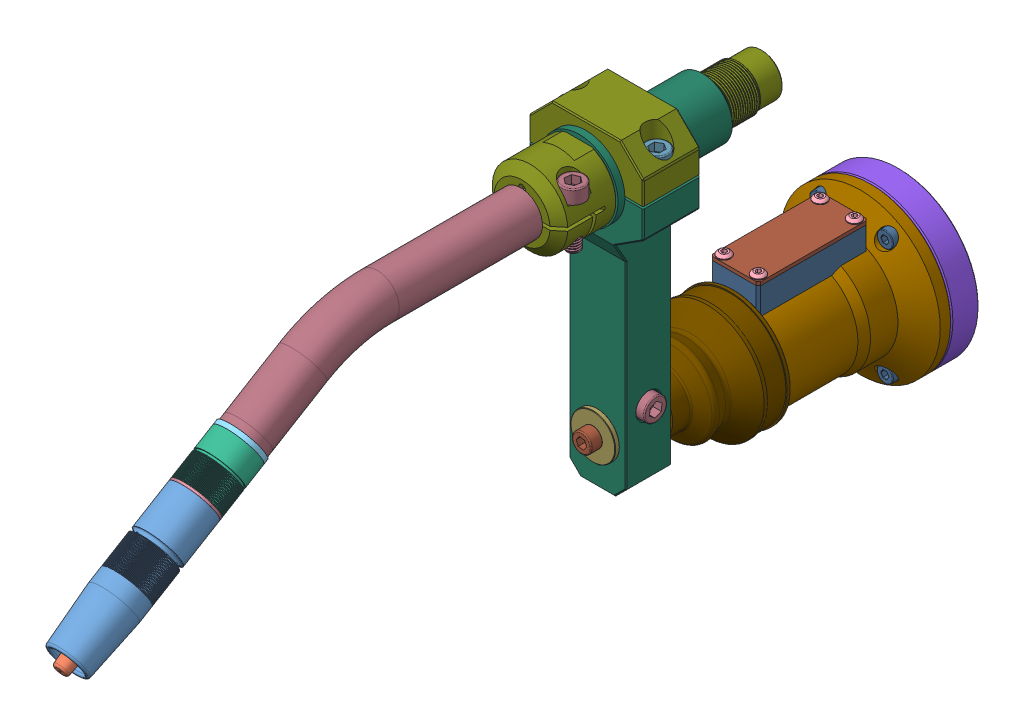
SolidWorks assembly 31度鵝頸，支架100.5L, configuration 默认. Lengths in mm.
Overall size (70 159.03 372.5).
47 component instances, 34 part files, 0 mates.
Components (placement in the parent):
- 31度鵝頸，支架100.5L-Part-1-1: 31度鵝頸，支架100.5L-Part-1 [默认] at (-1.3223 63.2513 288.8466) x (1 0 0) z (0 -0.857167 -0.515038) size (20 65.51 20)
- 31度鵝頸，支架100.5L-Part-2-1: 31度鵝頸，支架100.5L-Part-2 [默认] at (-1.3223 48.8303 312.8473) x (0 -0.515038 0.857167) z (-0.857167 0.441474 0.265264) size (40.5 8.7 8.7)
- 31度鵝頸，支架100.5L-Part-3-1: 31度鵝頸，支架100.5L-Part-3 [默认] at (-1.3223 56.2983 300.4183) x (1 0 0) z (0 -0.857167 -0.515038) size (15.5 21 15.5)
- 31度鵝頸，支架100.5L-Part-4-1: 31度鵝頸，支架100.5L-Part-4 [默认] at (-1.3223 63.7664 287.9894) x (0.857167 -0.441474 -0.265264) z (0 -0.515038 0.857167) size (20 20 1)
- 31度鵝頸，支架100.5L-Part-4-2: 31度鵝頸，支架100.5L-Part-4 [默认] at (-1.3223 63.2513 288.8466) x (1 0 0) z (0 0.515038 -0.857167) size (20 20 1)
- 31度鵝頸，支架100.5L-Part-5-1: 31度鵝頸，支架100.5L-Part-5 [默认] at (-1.3223 76.3848 266.9888) x (0 -0.515038 0.857167) z (-0.857167 0.441474 0.265264) size (38 20 20)
- 31度鵝頸，支架100.5L-Part-6-1: 31度鵝頸，支架100.5L-Part-6 [默认] at (-1.3223 76.3848 266.9888) x (0 -0.515038 0.857167) z (-0.857167 0.441474 0.265264) size (33.02 20 20)
- 31度鵝頸，支架100.5L-Part-7-1: 31度鵝頸，支架100.5L-Part-7 [默认] at (-1.3223 44.9675 319.276) x (0 0.515038 -0.857167) z (0.857167 0.441474 0.265264) size (80 14 16)
- 31度鵝頸，支架100.5L-Part-8-1: 31度鵝頸，支架100.5L-Part-8 [默认] at (-1.3223 100.8266 121.034) x (0 0 -1) z (1 0 0) size (2 12 12)
- 31度鵝頸，支架100.5L-Part-9-1: 31度鵝頸，支架100.5L-Part-9 [默认] at (-1.3223 0.3266 10.634) x (0 0 -1) z (-1 0 0) size (20 70 70)
- 31度鵝頸，支架100.5L-Part-10-1: 31度鵝頸，支架100.5L-Part-10 [默认] at (-16.0584 25.8771 1.634) x (-1 0 0) z (0 0 1) size (7 7 19)
- 31度鵝頸，支架100.5L-Part-10-2: 31度鵝頸，支架100.5L-Part-10 [默认] at (13.4416 25.8771 1.634) x (-1 0 0) z (0 0 1) size (7 7 19)
- 31度鵝頸，支架100.5L-Part-10-3: 31度鵝頸，支架100.5L-Part-10 [默认] at (-30.8084 0.3294 1.634) x (-1 0 0) z (0 0 1) size (7 7 19)
- 31度鵝頸，支架100.5L-Part-10-4: 31度鵝頸，支架100.5L-Part-10 [默认] at (13.4416 -25.2184 1.634) x (-1 0 0) z (0 0 1) size (7 7 19)
- 31度鵝頸，支架100.5L-Part-10-5: 31度鵝頸，支架100.5L-Part-10 [默认] at (-16.0584 -25.2184 1.634) x (-1 0 0) z (0 0 1) size (7 7 19)
- 31度鵝頸，支架100.5L-Part-11-1: 31度鵝頸，支架100.5L-Part-11 [默认] at (-1.3223 0.3266 119.534) x (0.923728 0.383049 0) z (0 0 -1) size (8.5 8.5 13.05)
- 31度鵝頸，支架100.5L-Part-12-1: 31度鵝頸，支架100.5L-Part-12 [默认] at (-1.3223 0.3266 114.534) x (-0.923728 -0.383049 0) z (0 0 -1) size (19.5 19.5 2)
- 31度鵝頸，支架100.5L-Part-13-1: 31度鵝頸，支架100.5L-Part-13 [默认] at (10.6777 113.8266 135.234) x (0.381849 0 0.924225) z (0 -1 0) size (10 10 26.16)
- 31度鵝頸，支架100.5L-Part-13-2: 31度鵝頸，支架100.5L-Part-13 [默认] at (14.1777 12.3266 102.534) x (0 -0.924225 -0.381849) z (-1 0 0) size (10 10 26.16)
- 31度鵝頸，支架100.5L-Part-14-1: 31度鵝頸，支架100.5L-Part-14 [默认] at (-19.8223 113.3266 105.034) x (1 0 0) z (0 -1 0) size (10 10 28.16)
- 31度鵝頸，支架100.5L-Part-14-2: 31度鵝頸，支架100.5L-Part-14 [默认] at (17.1777 114.3266 105.034) x (1 0 0) z (0 -1 0) size (10 10 28.16)
- 31度鵝頸，支架100.5L-Part-15-1: 31度鵝頸，支架100.5L-Part-15 [默认] at (-1.3223 -19.6734 117.534) x (-1 0 0) z (0 0 -1) size (50 120 25)
- 31度鵝頸，支架100.5L-Part-16-1: 31度鵝頸，支架100.5L-Part-16 [默认] at (-1.3223 -19.6734 117.534) x (-1 0 0) z (0 0 -1) size (50 20 25)
- 31度鵝頸，支架100.5L-Part-17-1: 31度鵝頸，支架100.5L-Part-17 [默认] at (-1.3223 -19.6734 117.534) x (-1 0 0) z (0 0 -1) size (12 12 12)
- 31度鵝頸，支架100.5L-Part-18-1: 31度鵝頸，支架100.5L-Part-18 [默认] at (-1.3223 0.3266 53.134) x (1 0 0) z (0 -1 0) size (50 38.5 50)
- 31度鵝頸，支架100.5L-Part-19-1: 31度鵝頸，支架100.5L-Part-19 [默认] at (-1.3223 -8.6734 110.134) x (1 0 0) z (0 1 0) size (3 15.7 3)
- 31度鵝頸，支架100.5L-Part-20-1: 31度鵝頸，支架100.5L-Part-20 [默认] at (-1.3223 0.3266 50.534) x (0 0 1) z (-1 0 0) size (61.8 31 31)
- 31度鵝頸，支架100.5L-Part-21-1: 31度鵝頸，支架100.5L-Part-21 [默认] at (-1.3223 20.3266 59.134) x (1 0 0) z (0 1 0) size (6.95 6.95 7)
- 31度鵝頸，支架100.5L-Part-21-2: 31度鵝頸，支架100.5L-Part-21 [默认] at (-1.3223 -19.6734 59.134) x (1 0 0) z (0 -1 0) size (6.95 6.95 7)
- 31度鵝頸，支架100.5L-Part-21-3: 31度鵝頸，支架100.5L-Part-21 [默认] at (-21.3223 0.3266 59.134) x (0 0 1) z (-1 0 0) size (6.95 6.95 7)
- 31度鵝頸，支架100.5L-Part-21-4: 31度鵝頸，支架100.5L-Part-21 [默认] at (18.6777 0.3266 59.134) x (0 0 -1) z (1 0 0) size (6.95 6.95 7)
- 31度鵝頸，支架100.5L-Part-22-1: 31度鵝頸，支架100.5L-Part-22 [默认] at (-8.8223 24.8266 49.634) size (5.7 9.6 5.7)
- 31度鵝頸，支架100.5L-Part-22-2: 31度鵝頸，支架100.5L-Part-22 [默认] at (6.1777 24.8266 49.634) size (5.7 9.6 5.7)
- 31度鵝頸，支架100.5L-Part-22-3: 31度鵝頸，支架100.5L-Part-22 [默认] at (-8.8223 24.8266 7.634) size (5.7 9.6 5.7)
- 31度鵝頸，支架100.5L-Part-22-4: 31度鵝頸，支架100.5L-Part-22 [默认] at (6.1777 24.8266 7.634) size (5.7 9.6 5.7)
- 31度鵝頸，支架100.5L-Part-23-1: 31度鵝頸，支架100.5L-Part-23 [默认] at (-1.3223 0.3266 65.634) x (-0.707107 -0.707107 0) z (0 0 -1) size (42 42 1)
- 31度鵝頸，支架100.5L-Part-24-1: 31度鵝頸，支架100.5L-Part-24 [默认] at (-1.3223 0.3266 65.634) x (-0.707107 -0.707107 0) z (0 0 -1) size (42 42 1)
- 31度鵝頸，支架100.5L-Part-25-1: 31度鵝頸，支架100.5L-Part-25 [默认] at (-1.3223 0.3266 53.634) size (42 42 11)
- 31度鵝頸，支架100.5L-Part-26-1: 31度鵝頸，支架100.5L-Part-26 [默认] at (-1.3223 0.3266 -1.366) x (0 0 -1) z (1 0 0) size (14.5 70 70)
- 31度鵝頸，支架100.5L-Part-27-1: 31度鵝頸，支架100.5L-Part-27 [默认] at (-1.3223 0.3266 -0.366) size (47 47 60)
- 31度鵝頸，支架100.5L-Part-28-1: 31度鵝頸，支架100.5L-Part-28 [默认] at (-1.3223 0.3266 -0.366) size (21.17 11.67 48)
- 31度鵝頸，支架100.5L-Part-29-1: 31度鵝頸，支架100.5L-Part-29 [默认] at (-1.3223 0.3266 -0.366) size (21 1.5 48)
- 31度鵝頸，支架100.5L-Part-30-1: 31度鵝頸，支架100.5L-Part-30 [默认] at (-1.3223 109.3266 144.534) x (-1 0 0) z (0 -1 0) size (3 12.5 3)
- 31度鵝頸，支架100.5L-Part-31-1: 31度鵝頸，支架100.5L-Part-31 [默认] at (-1.3223 100.8266 121.034) x (0 0 -1) z (1 0 0) size (127.05 42.81 19)
- 31度鵝頸，支架100.5L-Part-32-1: 31度鵝頸，支架100.5L-Part-32 [默认] at (-1.3223 100.8266 121.034) x (0 0 -1) z (1 0 0) size (148.04 38.42 16.86)
- 31度鵝頸，支架100.5L-Part-33-1: 31度鵝頸，支架100.5L-Part-33 [默认] at (-1.3223 100.8266 120.534) x (-0.546944 0.837169 0) z (0 0 -1) size (34 34 55)
- 31度鵝頸，支架100.5L-Part-34-1: 31度鵝頸，支架100.5L-Part-34 [默认] at (-1.3223 100.8266 145.534) x (0 1 0) z (-1 0 0) size (33 105 33)
